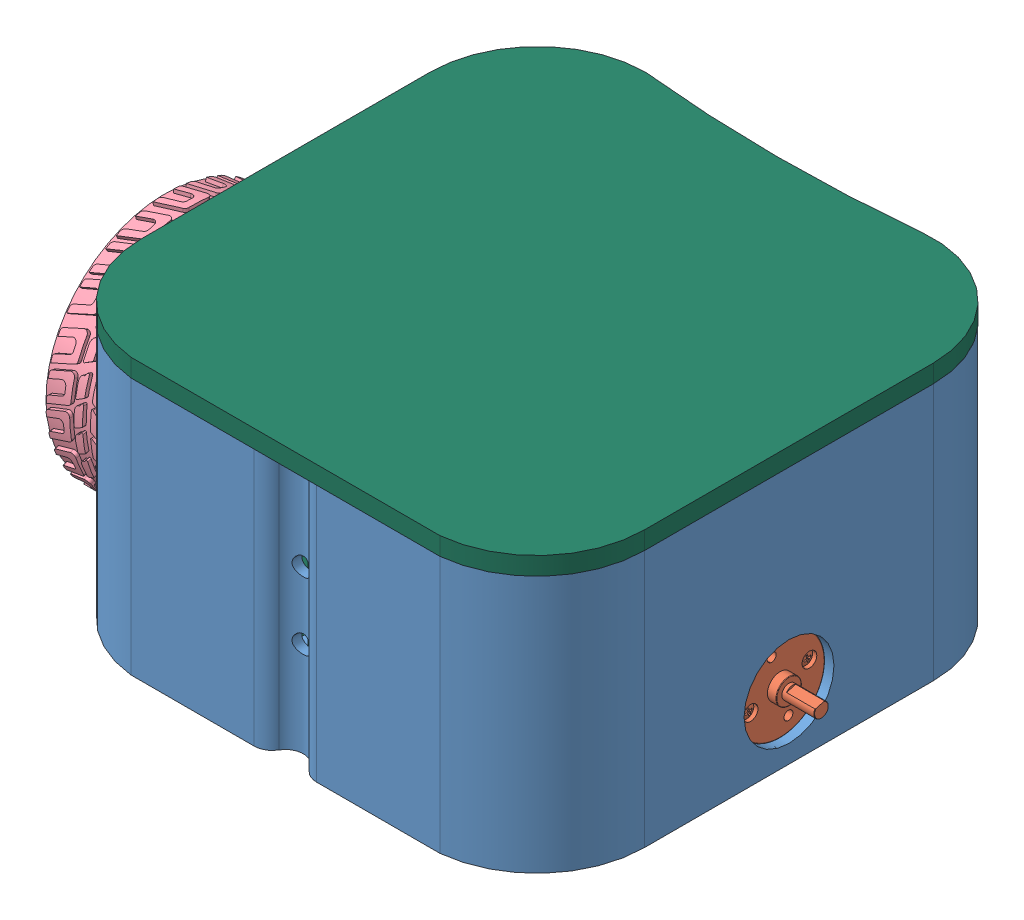
SolidWorks assembly Assem1, configuration Default. Lengths in mm.
Overall size (193.92 106.94 140.15).
40 component instances, 18 part files, 29 mates.
Components (placement in the parent):
- Base-1: Base [Default] at (79.9332 67.4802 109.8398) size (140 71.5 140.15)
- JGA25-372 24V Motor-1: JGA25-372 24V Motor [Ratio 171 & 226] at (12.9659 84.9802 109.8398) x (0 -0.051537 0.998671) z (0 -0.998671 -0.051537) size (25.02 71.1 25)
- wheeel-1: wheeel [Default] at (22.3528 137.773 120.8172) x (0 -0.759748 0.650217) z (0 -0.650217 -0.759748) size (68.01 32.89 68.01)
  - Part1-1: Part1 [Default] at (32.9715 20.0854 42.6668) size (55.88 32.89 55.88) (hidden)
  - Wheel-1: Wheel [Default] at (32.9715 45.9754 42.6668) x (1 0 0) z (0 -1 0) size (68.01 68.01 24.89) (hidden)
- JGA25-372 24V Motor-2: JGA25-372 24V Motor [Ratio 171 & 226] at (147.4332 84.9802 109.8398) x (0 0.273505 -0.961871) z (0 -0.961871 -0.273505) size (25.02 71.1 25)
- wheeel-2: wheeel [Default] at (131.0863 133.5777 86.4762) x (0 -0.893935 -0.448196) z (0 -0.448196 0.893935) size (68.01 32.89 68.01)
  - Part1-1: Part1 [Default] at (32.9715 20.0854 42.6668) size (55.88 32.89 55.88) (hidden)
  - Wheel-1: Wheel [Default] at (32.9715 45.9754 42.6668) x (1 0 0) z (0 -1 0) size (68.01 68.01 24.89) (hidden)
- Motor Drive Controller Module L298N-1: Motor Drive Controller Module L298N [Default] at (79.8332 115.5802 147.3398) x (0 0 1) z (1 0 0) size (47 28.4 44)
  - PCB_motor drive-1: PCB_motor drive [Default] x (1 0 0) z (0 1 0) size (47 44 1.6)
  - DISSIPATORE EXT_L298N-1: DISSIPATORE EXT_L298N [Default] at (15.5 14 0) x (-1 0 0) z (0 1 0) size (16 23.35 24.8)
  - L298N-1: L298N [Default] at (13.23 10.95 0) x (-1 0 0) z (0 1 0) size (9.91 20.2 25.1)
  - pin 8-2.54-1: pin 8-2.54 [Default] at (-17.73 4.14 11.73) x (0 0 -1) z (0 1 0) size (10.16 2.54 11.54)
  - pin 8-2.54_2-1: pin 8-2.54_2 [Default] at (-17.73 4.14 14.48) x (1 0 0) z (0 1 0) size (5.08 2.54 11.54)
  - pin 8-2.54_2-2: pin 8-2.54_2 [Default] at (-17.73 4.14 1.23) x (1 0 0) z (0 1 0) size (5.08 2.54 11.54)
  - pin 8-2.54_2-3: pin 8-2.54_2 [Default] at (-10.73 4.14 -9.69) x (0 0 -1) z (0 1 0) size (5.08 2.54 11.54)
  - TE_1776244-2-1: TE_1776244-2 [Default] at (-16.5 1.6 -11) x (0 0 1) z (-1 0 0) size (16.16 13.5 7.5)
  - TE_1776244-2_2-1: TE_1776244-2_2 [Default] at (-6 1.6 -18.2) x (-1 0 0) z (0 0 -1) size (11.16 13.5 7.5)
  - TE_1776244-2_2-2: TE_1776244-2_2 [Default] at (-6 1.6 18.2) size (11.16 13.5 7.5)
  - PIN BLOCCO DISSIPATORE EXT-1: PIN BLOCCO DISSIPATORE EXT [Default] at (17.1 -1.9 9.175) x (1 0 0) z (0 1 0) size (1 1 10)
  - PIN BLOCCO DISSIPATORE EXT-2: PIN BLOCCO DISSIPATORE EXT [Default] at (17.1 -1.9 -9.175) x (1 0 0) z (0 1 0) size (1 1 10)
- Goouuu-ESP32 Development Board-1: Goouuu-ESP32 Development Board [Default] at (79.9332 101.4302 51.3398) x (-1 0 0) z (0 -1 0) size (27.94 13.14 55.58)
- battary-1: battary [Default] at (133.4332 128.2802 76.3398) x (0.99715 0.075442 0) z (0.075442 -0.99715 0) size (18.5 67 18.5)
- battary-2: battary [Default] at (133.4332 109.4802 76.3398) x (0.969694 0.244324 0) z (0.244324 -0.969694 0) size (18.5 67 18.5)
- battary-3: battary [Default] at (26.4332 128.2802 76.3398) x (1 0 0) z (0 -1 0) size (18.5 67 18.5)
- battary-4: battary [Default] at (26.4332 109.4802 76.3398) x (1 0 0) z (0 -1 0) size (18.5 67 18.5)
- wheeel-3: wheeel [Default] at (29.1192 32.1974 98.815) x (0 0.760333 -0.649534) z (0 0.649534 0.760333) size (68.01 32.89 68.01)
  - Part1-1: Part1 [Default] at (32.9715 20.0854 42.6668) size (55.88 32.89 55.88) (hidden)
  - Wheel-1: Wheel [Default] at (32.9715 45.9754 42.6668) x (1 0 0) z (0 -1 0) size (68.01 68.01 24.89) (hidden)
- cover-1: cover [Default] at (69.3971 143.9802 107.7431) x (-1 0 0) z (0 0 1) size (140 65 140.15)
- motor holder-1: motor holder [Default] at (146.9332 84.9802 109.8398) x (0 0 1) z (0 -1 0) size (53 32 25.5)
- vl53l0x-1: vl53l0x [Default] at (79.9867 128.9604 46.4779) x (1 0 0) z (0 1 0) size (25 11.3 11)
  - vl53l0x_PCB-1: vl53l0x_PCB [Default] at origin size (25 3 11)
  - pin_header-1: pin_header [Default] at (-6.5 -2.54 4) size (2.54 11.3 2.54)
  - pin_header-2: pin_header [Default] at (-3.96 -2.54 4) size (2.54 11.3 2.54)
  - pin_header-3: pin_header [Default] at (-1.42 -2.54 4) size (2.54 11.3 2.54)
  - pin_header-4: pin_header [Default] at (1.12 -2.54 4) size (2.54 11.3 2.54)
  - pin_header-5: pin_header [Default] at (3.66 -2.54 4) size (2.54 11.3 2.54)
  - pin_header-6: pin_header [Default] at (6.2 -2.54 4) size (2.54 11.3 2.54)
Mates (geometry in assembly coordinates):
- Concentric7: concentric: cylinder of JGA25-372 24V Motor-1 through (-4.191 84.9802 109.8398) axis (1 0 0) radius 2; cylinder of wheeel-1/Part1-1 through (9.2674 84.9802 109.8398) axis (-1 0 0) radius 2
- Concentric8: concentric: cylinder of JGA25-372 24V Motor-2 through (164.5901 84.9802 109.8398) axis (-1 0 0) radius 2; cylinder of wheeel-2/Part1-1 through (144.1717 84.9802 109.8398) axis (1 0 0) radius 2
- Concentric9: concentric: cylinder of Base-1 through (149.9332 84.9802 109.8398) axis (-1 0 0) radius 12.5; cylinder of JGA25-372 24V Motor-2 through (-852.5668 84.9802 109.8398) axis (-1 0 0) radius 12.5
- Concentric10: concentric: cylinder of Base-1 through (149.9332 84.9802 109.8398) axis (-1 0 0) radius 12.5; cylinder of JGA25-372 24V Motor-1 through (1012.9659 84.9802 109.8398) axis (1 0 0) radius 12.5
- Coincident26: coincident: plane of battary-1 through (133.4332 128.2802 143.3398) normal (0 0 1); plane of battary-2 through (133.4332 109.4802 143.3398) normal (0 0 1)
- Concentric23: concentric: cylinder of Base-1 through (133.4332 128.2802 65.8398) axis (0 0 1) radius 9.4; cylinder of battary-1 through (133.4332 128.2802 143.3398) axis (0 0 -1) radius 9.25
- Concentric24: concentric: cylinder of Base-1 through (133.4332 109.4802 65.8398) axis (0 0 1) radius 9.4; cylinder of battary-2 through (133.4332 109.4802 143.3398) axis (0 0 -1) radius 9.25
- Distance2: distance = 13.5 mm: plane of battary-1 through (133.4332 128.2802 76.3398) normal (0 0 -1); plane of Base-1 through (146.9332 138.9802 89.8398) normal (0 0 -1)
- Concentric30: concentric: cylinder of Base-1 through (26.4332 128.2802 65.8398) axis (0 0 1) radius 9.4; cylinder of battary-3 through (26.4332 128.2802 143.3398) axis (0 0 -1) radius 9.25
- Coincident29: coincident: plane of battary-1 through (133.4332 128.2802 143.3398) normal (0 0 1); plane of battary-3 through (26.4332 128.2802 143.3398) normal (0 0 1)
- Concentric31: concentric: cylinder of Base-1 through (26.4332 109.4802 65.8398) axis (0 0 1) radius 9.4; cylinder of battary-4 through (26.4332 109.4802 143.3398) axis (0 0 -1) radius 9.25
- Coincident32: coincident: plane of Base-1 through (79.9332 73.9802 179.8398) normal (0 1 0); plane of Goouuu-ESP32 Development Board-1 through (93.8832 73.9802 49.7398) normal (0 -1 0)
- Parallel2: parallel: plane of Base-1 through (34.8034 73.9802 176.8398) normal (0 0 -1); plane of Goouuu-ESP32 Development Board-1 through (88.9332 103.3802 46.7398) normal (0 0 -1)
- Coincident30: coincident: circle of battary-3; plane of battary-4 through (26.4332 109.4802 143.3398) normal (0 0 1)
- Coincident34: coincident: plane of Base-1 through (61.0332 113.9802 129.8398) normal (0 1 0); plane of Motor Drive Controller Module L298N-1/PCB_motor drive-1 through (79.8332 113.9802 147.3398) normal (0 -1 0)
- Concentric34: concentric: cylinder of Base-1 through (98.8332 113.9802 129.8398) axis (0 -1 0) radius 2; cylinder of Motor Drive Controller Module L298N-1/PCB_motor drive-1 through (98.8332 114.0802 129.8398) axis (0 1 0) radius 1.5
- Concentric35: concentric: cylinder of Base-1 through (61.0332 113.9802 129.8398) axis (0 -1 0) radius 2; cylinder of Motor Drive Controller Module L298N-1/PCB_motor drive-1 through (61.0332 114.0802 129.8398) axis (0 1 0) radius 1.5
- Concentric36: concentric: cylinder of JGA25-372 24V Motor-1 through (-4.191 84.9802 109.8398) axis (1 0 0) radius 2; cylinder of wheeel-3/Part1-1 through (16.0338 84.9802 109.8398) axis (-1 0 0) radius 2
- Concentric38: concentric: cylinder of JGA25-372 24V Motor-2 through (-852.5668 84.9802 109.8398) axis (-1 0 0) radius 12.5; cylinder of motor holder-1 through (114.9332 84.9802 109.8398) axis (1 0 0) radius 12.5
- Coincident36: coincident: plane of Base-1 through (79.9332 73.9802 179.8398) normal (0 1 0); plane of motor holder-1 through (146.9332 73.9802 109.8398) normal (0 -1 0)
- Coincident37: coincident: plane of Base-1 through (119.9332 142.4802 129.3398) normal (-1 0 0); plane of motor holder-1 through (119.9332 73.9802 95.3398) normal (1 0 0)
- Concentric40: concentric: cylinder of Base-1 through (27.9332 63.9802 161.8398) axis (0 1 0) radius 2.5; cylinder of cover-1 through (27.9332 78.9802 161.8398) axis (0 1 0) radius 2
- Concentric41: concentric: cylinder of Base-1 through (131.9332 63.9802 57.8398) axis (0 1 0) radius 2.5; cylinder of cover-1 through (131.9332 78.9802 57.8398) axis (0 1 0) radius 2
- Concentric42: concentric: cylinder of Base-1 through (27.9332 63.9802 57.8398) axis (0 1 0) radius 2.5; cylinder of cover-1 through (27.9332 78.9802 57.8398) axis (0 1 0) radius 2
- Concentric43: concentric: cylinder of Base-1 through (131.9332 63.9802 161.8398) axis (0 1 0) radius 2.5; cylinder of cover-1 through (131.9332 78.9802 161.8398) axis (0 1 0) radius 2
- Coincident38: coincident: plane of Base-1 through (79.9332 138.9802 109.8398) normal (0 1 0); plane of cover-1 through (79.1369 138.9802 -334.1548) normal (0 -1 0)
- Parallel3: parallel: plane of Base-1 through (49.9332 63.9802 84.8398) normal (0 0 -1); plane of vl53l0x-1/vl53l0x_PCB-1 through (70.2367 128.9604 46.4779) normal (0 0 1)
- Parallel4: parallel: plane of Base-1 through (79.9332 73.9802 179.8398) normal (0 1 0); plane of vl53l0x-1/vl53l0x_PCB-1 through (87.9867 123.4604 45.4779) normal (0 -1 0)
- Tangent1: tangent: cylinder of Base-1 through (81.4402 73.9802 -360.266) axis (0 1 0) radius 404.7439; plane of vl53l0x-1/vl53l0x_PCB-1 through (79.9867 128.9604 44.4779) normal (0 0 -1)
